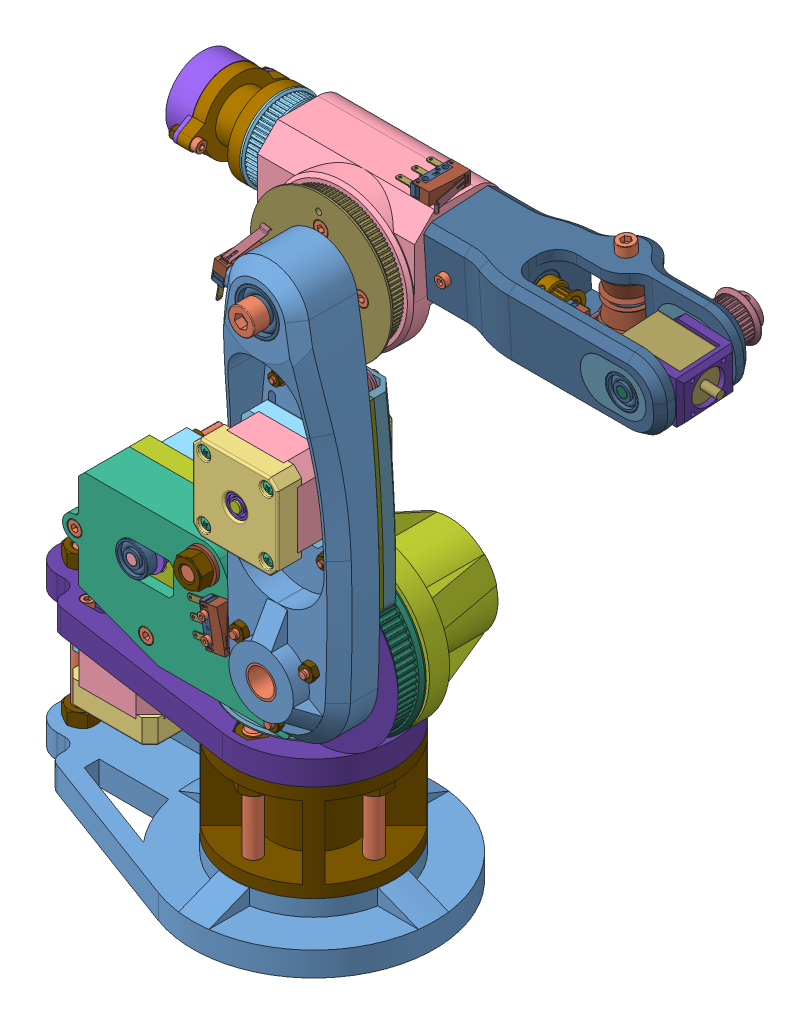
SolidWorks assembly Assem4_v2, configuration Default. Lengths in mm. (continued)
Mates (geometry in assembly coordinates): (continued)
- Coincident177: coincident: plane of Pulley100TBase-2 through (106.8987 -12.6787 52.4417) normal (0 -1 0); plane of thrust ball bearing_68_iso-1 through (106.6815 -12.6787 62.7394) normal (0 1 0)
- Coincident178: coincident: plane of Baseplate-1 through (106.8987 -29.6787 52.4417) normal (0 -1 0); plane of NEMA 17 kiinalaiset-2/Tapa-1 through (25.5987 -29.6787 52.4417) normal (0 1 0)
- Concentric171: concentric: cylinder of Baseplate-1 through (10.0987 -41.6995 36.9417) axis (0 1 0) radius 1.75; cylinder of NEMA 17 kiinalaiset-2/Tapa-1 through (10.0987 -34.1787 36.9417) axis (0 1 0) radius 1.5
- Concentric172: concentric: cylinder of Baseplate-1 through (41.0987 -41.6995 67.9417) axis (0 1 0) radius 1.75; cylinder of NEMA 17 kiinalaiset-2/Tapa-1 through (41.0987 -34.1787 67.9417) axis (0 1 0) radius 1.5
- Concentric173: concentric: cylinder of Baseplate-1 through (10.0987 -41.6995 36.9417) axis (0 1 0) radius 1.75; cylinder of socket head cap screw_iso-60 through (10.0987 12.0713 36.9417) axis (0 1 0) radius 2.75
- Coincident179: coincident: plane of Baseplate-1 through (18.0987 -22.6787 36.9417) normal (0 1 0); plane of socket head cap screw_iso-60 through (12.7426 -22.6787 36.1851) normal (0 -1 0)
- Concentric174: concentric: cylinder of Baseplate-1 through (10.0987 -41.6995 67.9417) axis (0 1 0) radius 1.75; cylinder of socket head cap screw_iso-61 through (10.0987 12.0713 67.9417) axis (0 1 0) radius 2.75
- Coincident180: coincident: plane of Baseplate-1 through (18.0987 -22.6787 67.9417) normal (0 1 0); plane of socket head cap screw_iso-61 through (12.8487 -22.6787 67.9417) normal (0 -1 0)
- Concentric175: concentric: cylinder of Baseplate-1 through (41.0987 -22.6787 36.9417) axis (0 1 0) radius 3; cylinder of socket head cap screw_iso-62 through (41.0987 12.0713 36.9417) axis (0 1 0) radius 2.75
- Coincident181: coincident: plane of Baseplate-1 through (49.0987 -22.6787 36.9417) normal (0 1 0); plane of socket head cap screw_iso-62 through (43.8487 -22.6787 36.9417) normal (0 -1 0)
- Concentric176: concentric: cylinder of Baseplate-1 through (41.0987 -22.6787 67.9417) axis (0 1 0) radius 3; cylinder of socket head cap screw_iso-63 through (41.0987 12.0713 67.9417) axis (0 1 0) radius 2.75
- Coincident182: coincident: plane of Baseplate-1 through (49.0987 -22.6787 67.9417) normal (0 1 0); plane of socket head cap screw_iso-63 through (43.8487 -22.6787 67.9417) normal (0 -1 0)
- Concentric177: concentric: cylinder of NEMA 17 kiinalaiset-2/Eje-1 through (25.5987 -7.6787 52.4417) axis (0 -1 0) radius 2.5; cylinder of GT2_16T_13x14-3 through (25.5987 -20.2487 52.4417) axis (0 1 0) radius 2.5
- Coincident183: coincident: plane of Pulley100TBase-2 through (106.8987 -14.0787 52.4417) normal (0 1 0); plane of GT2_16T_13x14-3 through (25.5987 -14.0787 52.4417) normal (0 1 0)
- Concentric178: concentric: cylinder of Bottom support-1 through (106.8987 -110.9924 22.4417) axis (0 1 0) radius 4; cylinder of socket head cap screw_iso-65 through (106.8987 -129.4287 22.4417) axis (0 -1 0) radius 6.5
- Coincident184: coincident: plane of Bottom support-1 through (106.8987 -89.6787 22.4417) normal (0 -1 0); plane of socket head cap screw_iso-65 through (100.3987 -89.6787 22.4417) normal (0 1 0)
- Concentric179: concentric: cylinder of Bottom support-1 through (76.8987 -89.6787 52.4417) axis (0 -1 0) radius 7.5; cylinder of socket head cap screw_iso-66 through (76.8987 -129.4287 52.4417) axis (0 -1 0) radius 6.5
- Coincident185: coincident: plane of Bottom support-1 through (76.8987 -89.6787 52.4417) normal (0 -1 0); plane of socket head cap screw_iso-66 through (70.3987 -89.6787 52.4417) normal (0 1 0)
- Concentric180: concentric: cylinder of Bottom support-1 through (106.8987 -110.9924 82.4417) axis (0 1 0) radius 4; cylinder of socket head cap screw_iso-67 through (106.8987 -129.4287 82.4417) axis (0 -1 0) radius 6.5
- Coincident186: coincident: plane of Bottom support-1 through (106.8987 -89.6787 82.4417) normal (0 -1 0); plane of socket head cap screw_iso-67 through (100.3987 -89.6787 82.4417) normal (0 1 0)
- Concentric181: concentric: cylinder of Bottom support-1 through (136.8987 -110.9924 52.4417) axis (0 1 0) radius 4; cylinder of socket head cap screw_iso-68 through (136.8987 -129.4287 52.4417) axis (0 -1 0) radius 6.5
- Coincident187: coincident: plane of Bottom support-1 through (136.8987 -89.6787 52.4417) normal (0 -1 0); plane of socket head cap screw_iso-68 through (130.3987 -89.6787 52.4417) normal (0 1 0)
- Concentric182: concentric: cylinder of socket head cap screw_iso-65 through (106.8987 -129.4287 22.4417) axis (0 -1 0) radius 4; cylinder of hex nut style 1 gradeab_iso-26 through (106.8987 -19.4412 22.4417) axis (0 -1 0) radius 4
- Concentric183: concentric: cylinder of socket head cap screw_iso-68 through (136.8987 -129.4287 52.4417) axis (0 -1 0) radius 4; cylinder of hex nut style 1 gradeab_iso-27 through (136.8987 -19.4412 52.4417) axis (0 -1 0) radius 4
- Concentric184: concentric: cylinder of socket head cap screw_iso-67 through (106.8987 -129.4287 82.4417) axis (0 -1 0) radius 4; cylinder of hex nut style 1 gradeab_iso-28 through (106.8987 -19.4412 82.4417) axis (0 -1 0) radius 4
- Concentric185: concentric: cylinder of socket head cap screw_iso-66 through (76.8987 -129.4287 52.4417) axis (0 -1 0) radius 4; cylinder of hex nut style 1 gradeab_iso-29 through (76.8987 -18.4412 52.4417) axis (0 -1 0) radius 4
- Concentric186: concentric: cylinder of Baseplate-1 through (106.8987 -42.9924 82.4417) axis (0 1 0) radius 4; cylinder of hex nut style 1 gradeab_iso-30 through (106.8987 -45.9162 82.4417) axis (0 1 0) radius 4
- Coincident188: coincident: plane of Baseplate-1 through (106.8987 -27.6787 52.4417) normal (0 1 0); plane of hex nut style 1 gradeab_iso-30 through (103.146 -27.6787 75.9417) normal (0 -1 0)
- Concentric187: concentric: cylinder of socket head cap screw_iso-68 through (136.8987 -129.4287 52.4417) axis (0 -1 0) radius 4; cylinder of hex nut style 1 gradeab_iso-31 through (136.8987 -2.6412 52.4417) axis (0 -1 0) radius 4
- Concentric188: concentric: cylinder of Baseplate-1 through (106.8987 -42.9924 22.4417) axis (0 1 0) radius 4; cylinder of hex nut style 1 gradeab_iso-32 through (106.8987 -45.9162 22.4417) axis (0 1 0) radius 4
- Coincident189: coincident: plane of Baseplate-1 through (106.8987 -27.6787 52.4417) normal (0 1 0); plane of hex nut style 1 gradeab_iso-32 through (110.6515 -27.6787 28.9417) normal (0 -1 0)
- Concentric189: concentric: cylinder of socket head cap screw_iso-66 through (76.8987 -129.4287 52.4417) axis (0 -1 0) radius 4; cylinder of hex nut style 1 gradeab_iso-33 through (76.8987 -2.6412 52.4417) axis (0 -1 0) radius 4
- Coincident190: coincident: plane of Bottom Tube-1 through (106.8987 -37.6787 52.4417) normal (0 -1 0); plane of hex nut style 1 gradeab_iso-28 through (106.8987 -37.6787 89.9473) normal (0 1 0)
- Coincident191: coincident: plane of hex nut style 1 gradeab_iso-26 through (106.8987 -37.6787 29.9473) normal (0 1 0); plane of Bottom Tube-1 through (106.8987 -37.6787 52.4417) normal (0 -1 0)
- Coincident192: coincident: plane of Bottom Tube-1 through (106.8987 -37.6787 52.4417) normal (0 -1 0); plane of hex nut style 1 gradeab_iso-27 through (136.8987 -37.6787 59.9473) normal (0 1 0)
- Coincident193: coincident: plane of Baseplate-1 through (143.3987 -27.6787 56.1945) normal (-1 0 0); plane of hex nut style 1 gradeab_iso-31 through (143.3987 -20.8787 56.1945) normal (1 0 0)
- Coincident194: coincident: plane of Baseplate-1 through (106.8987 -27.6787 52.4417) normal (0 1 0); plane of hex nut style 1 gradeab_iso-31 through (136.8987 -27.6787 59.9473) normal (0 -1 0)
- Coincident195: coincident: plane of Baseplate-1 through (114.4043 -27.6787 22.4417) normal (-0.866025 0 0.5); plane of hex nut style 1 gradeab_iso-32 through (114.4043 -27.6787 22.4417) normal (0.866025 0 -0.5)
- Coincident196: coincident: plane of Baseplate-1 through (70.3987 -27.6787 56.1945) normal (0.5 0 -0.866025); plane of hex nut style 1 gradeab_iso-33 through (76.8987 -20.8787 59.9473) normal (-0.5 0 0.866025)
- Coincident197: coincident: plane of Baseplate-1 through (106.8987 -27.6787 52.4417) normal (0 1 0); plane of hex nut style 1 gradeab_iso-33 through (76.8987 -27.6787 59.9473) normal (0 -1 0)
- Coincident198: coincident: plane of Baseplate-1 through (103.146 -27.6787 75.9417) normal (0.866025 0 0.5); plane of hex nut style 1 gradeab_iso-30 through (103.146 -27.6787 75.9417) normal (-0.866025 0 -0.5)
- Concentric190: concentric: cylinder of Nema 14 stepper-1 through (113.8987 155.7922 35.8417) axis (-1 0 0) radius 1.5; cylinder of socket head cap screw_iso-42 through (69.6487 155.7922 35.8417) axis (-1 0 0) radius 1.5
- Concentric191: concentric: cylinder of Bottom support-1 through (-8.1013 -75.7993 52.4417) axis (0 -1 0) radius 4.2; cylinder of hex bolt gradeab_iso-2 through (-8.1013 -98.9787 52.4417) axis (0 -1 0) radius 6.5
- Coincident201: coincident: plane of Bottom support-1 through (106.8987 -93.6787 52.4417) normal (0 -1 0); plane of hex bolt gradeab_iso-2 through (-15.6068 -93.6787 52.4417) normal (0 1 0)
- Coincident202: coincident: plane of Bottom support-1 through (-11.854 -93.6787 45.9417) normal (0 0 1); plane of hex bolt gradeab_iso-2 through (-11.854 -93.6787 45.9417) normal (0 0 -1)
- Concentric192: concentric: cylinder of hex bolt gradeab_iso-2 through (-8.1013 -98.9787 52.4417) axis (0 -1 0) radius 4; cylinder of hex nut style 1 gradeab_iso-35 through (-8.1013 -62.6412 52.4417) axis (0 -1 0) radius 4
- Concentric193: concentric: cylinder of hex bolt gradeab_iso-2 through (-8.1013 -98.9787 52.4417) axis (0 -1 0) radius 4; cylinder of hex nut style 1 gradeab_iso-36 through (-8.1013 -13.4412 52.4417) axis (0 -1 0) radius 4
- Concentric194: concentric: cylinder of hex bolt gradeab_iso-2 through (-8.1013 -98.9787 52.4417) axis (0 -1 0) radius 4; cylinder of hex nut style 1 gradeab_iso-37 through (-8.1013 5.3588 52.4417) axis (0 -1 0) radius 4
- Coincident203: coincident: plane of Bottom support-1 through (106.8987 -87.6787 52.4417) normal (0 1 0); plane of hex nut style 1 gradeab_iso-35 through (-8.1013 -87.6787 59.9473) normal (0 -1 0)
- Coincident204: coincident: plane of Baseplate-1 through (106.8987 -19.6787 52.4417) normal (0 1 0); plane of hex nut style 1 gradeab_iso-37 through (-8.1013 -19.6787 59.9473) normal (0 -1 0)
- Coincident206: coincident: plane of Baseplate-1 through (106.8987 -31.6787 52.4417) normal (0 -1 0); plane of hex nut style 1 gradeab_iso-36 through (-8.1013 -31.6787 59.9473) normal (0 1 0)
- Concentric196: concentric: cylinder of Nema 17 planetary 5 to 1 gearbox-1 through (59.3987 35.6213 65.4417) axis (0 0 -1) radius 3; cylinder of HTD pulley adapter-1 through (59.3987 35.6213 65.4417) axis (0 0 -1) radius 3
- Coincident208: coincident: plane of Nema 17 planetary 5 to 1 gearbox-1 through (59.3987 35.6213 65.4417) normal (0 0 1); plane of HTD pulley adapter-1 through (59.3987 35.6213 65.4417) normal (0 0 -1)
- Concentric200: concentric: cylinder of Nema 17 planetary 5 to 1 gearbox-1 through (59.3987 35.6213 49.4417) axis (0 0 -1) radius 11; cylinder of Motor1 spacer-1 through (59.3987 35.6213 62.4417) axis (0 0 -1) radius 9
- Concentric201: concentric: cylinder of Nema 17 planetary 5 to 1 gearbox-1 through (49.4992 45.5208 42.4417) axis (0 0 1) radius 1.5; cylinder of Motor1 spacer-1 through (49.4992 45.5208 42.7748) axis (0 0 1) radius 1.65
- Coincident214: coincident: plane of Nema 17 planetary 5 to 1 gearbox-1 through (59.3987 35.6213 47.4417) normal (0 0 1); plane of Motor1 spacer-1 through (59.3987 35.6213 47.4417) normal (0 0 -1)
- Concentric202: concentric: cylinder of Motor1 spacer-1 through (49.4992 45.5208 42.7748) axis (0 0 1) radius 1.65; cylinder of socket head cap screw_iso-70 through (49.4992 45.5208 89.1917) axis (0 0 1) radius 2.75
- Coincident215: coincident: plane of Motor1 spacer-1 through (59.3987 35.6213 54.4417) normal (0 0 1); plane of socket head cap screw_iso-70 through (49.4992 48.2708 54.4417) normal (0 0 -1)
- Concentric203: concentric: cylinder of Motor1 spacer-1 through (69.2982 45.5208 42.7748) axis (0 0 1) radius 1.65; cylinder of socket head cap screw_iso-71 through (69.2982 45.5208 89.1917) axis (0 0 1) radius 2.75
- Coincident216: coincident: plane of Motor1 spacer-1 through (59.3987 35.6213 54.4417) normal (0 0 1); plane of socket head cap screw_iso-71 through (69.2982 48.2708 54.4417) normal (0 0 -1)
- Concentric204: concentric: cylinder of Motor1 spacer-1 through (69.2982 25.7218 42.7748) axis (0 0 1) radius 1.65; cylinder of socket head cap screw_iso-72 through (69.2982 25.7218 89.1917) axis (0 0 1) radius 2.75
- Coincident217: coincident: plane of Motor1 spacer-1 through (59.3987 35.6213 54.4417) normal (0 0 1); plane of socket head cap screw_iso-72 through (69.2982 28.4718 54.4417) normal (0 0 -1)
- Concentric205: concentric: cylinder of Motor1 spacer-1 through (49.4992 25.7218 42.7748) axis (0 0 1) radius 1.65; cylinder of socket head cap screw_iso-73 through (49.4992 25.7218 89.1917) axis (0 0 1) radius 2.75
- Coincident218: coincident: plane of Motor1 spacer-1 through (59.3987 35.6213 54.4417) normal (0 0 1); plane of socket head cap screw_iso-73 through (49.4992 28.4718 54.4417) normal (0 0 -1)
- Concentric212: concentric: cylinder of Motor1 spacer-1 through (76.8987 53.1213 62.4417) axis (0 0 -1) radius 2; cylinder of hex nut style 1 gradeab_iso-39 through (76.8987 53.1213 69.2792) axis (0 0 -1) radius 2
- Coincident226: coincident: plane of Motor1 spacer-1 through (59.3987 35.6213 47.4417) normal (0 0 -1); plane of hex nut style 1 gradeab_iso-39 through (78.4468 49.3881 47.4417) normal (0 0 1)
- Concentric213: concentric: cylinder of Motor1 spacer-1 through (41.8987 53.1213 62.4417) axis (0 0 -1) radius 2; cylinder of hex nut style 1 gradeab_iso-40 through (41.8987 53.1213 69.2792) axis (0 0 -1) radius 2
- Coincident227: coincident: plane of Motor1 spacer-1 through (59.3987 35.6213 47.4417) normal (0 0 -1); plane of hex nut style 1 gradeab_iso-40 through (43.4468 49.3881 47.4417) normal (0 0 1)
- Concentric214: concentric: cylinder of Motor1 spacer-1 through (41.8987 18.1213 62.4417) axis (0 0 -1) radius 2; cylinder of hex nut style 1 gradeab_iso-41 through (41.8987 18.1213 69.2792) axis (0 0 -1) radius 2
- Coincident228: coincident: plane of Motor1 spacer-1 through (59.3987 35.6213 47.4417) normal (0 0 -1); plane of hex nut style 1 gradeab_iso-41 through (43.4468 14.3881 47.4417) normal (0 0 1)
- Concentric215: concentric: cylinder of Motor1 spacer-1 through (76.8987 18.1213 62.4417) axis (0 0 -1) radius 2; cylinder of hex nut style 1 gradeab_iso-42 through (76.8987 18.1213 69.2792) axis (0 0 -1) radius 2
- Coincident229: coincident: plane of Motor1 spacer-1 through (59.3987 35.6213 47.4417) normal (0 0 -1); plane of hex nut style 1 gradeab_iso-42 through (78.4468 14.3881 47.4417) normal (0 0 1)
- Concentric216: concentric: cylinder of socket head cap screw_iso-54 through (30.3987 34.1213 126.3917) axis (0 0 1) radius 2; cylinder of Basewall cover v2-1 through (30.3987 34.1213 66.7849) axis (0 0 1) radius 2
- Concentric217: concentric: cylinder of socket head cap screw_iso-50 through (65.8987 5.6213 126.3917) axis (0 0 1) radius 2; cylinder of Basewall cover v2-1 through (65.8987 5.6213 94.6417) axis (0 0 -1) radius 2.1
- Coincident231: coincident: plane of socket head cap screw_iso-54 through (29.6963 37.5501 90.6417) normal (0 0 -1); plane of Basewall cover v2-1 through (30.3987 34.1213 90.6417) normal (0 0 1)
- Coincident232: coincident: plane of socket head cap screw_iso-50 through (67.7589 8.5861 90.6417) normal (0 0 -1); plane of Basewall cover v2-1 through (65.8987 5.6213 90.6417) normal (0 0 1)
- Concentric220: concentric: cylinder of socket head cap screw_iso-23 through (94.3987 50.6213 22.6917) axis (0 0 -1) radius 4; cylinder of plain washer normal grade a_iso-20 through (94.3987 50.6213 129.5667) axis (0 0 1) radius 4.2
- Coincident233: coincident: plane of plain washer normal grade a_iso-20 through (90.8481 52.8648 94.6417) normal (0 0 -1); plane of Basewall cover v2-1 through (133.7832 -1.1274 94.6417) normal (0 0 1)
- Concentric221: concentric: cylinder of socket head cap screw_iso-36 through (101.319 35.6213 134.5917) axis (0 0 1) radius 1; cylinder of Basewall cover v2-1 through (101.319 35.6213 86.8133) axis (0 0 1) radius 1
- Concentric222: concentric: cylinder of socket head cap screw_iso-37 through (103.0555 25.7732 134.5917) axis (0 0 1) radius 1; cylinder of Basewall cover v2-1 through (103.0555 25.7732 86.8133) axis (0 0 1) radius 1
- Coincident234: coincident: plane of ? through (103.04 32.6599 94.6417) normal (0 0 -1); plane of Basewall cover v2-1 through (133.7832 -1.1274 94.6417) normal (0 0 1)
- Concentric223: concentric: cylinder of 90mm aluputki-1 through (144.3987 35.6213 116.0417) axis (0 0 -1) radius 7.5; cylinder of BaseWall_2_v2-1 through (144.3987 35.6213 72.4417) axis (0 0 -1) radius 10
- Concentric224: concentric: cylinder of Pulley100TBase-2 through (106.8987 -14.0787 52.4417) axis (0 1 0) radius 7.5; cylinder of BaseWall_2_v2-1 through (106.8987 40.6213 52.4417) axis (0 -1 0) radius 7.65
- Coincident235: coincident: plane of angular contact ball bearing_68_iso-5 through (152.6194 47.2916 63.4417) normal (0 0 -1); plane of BaseWall_2_v2-1 through (144.3987 35.6213 63.4417) normal (0 0 1)
- Coincident236: coincident: plane of angular contact ball bearing_68_iso-6 through (145.4625 51.2852 31.4417) normal (0 0 1); plane of BaseWall_2_v2-1 through (144.3987 35.6213 31.4417) normal (0 0 -1)
- Coincident237: coincident: plane of Bottom spacer-1 through (106.8987 -4.3787 52.4417) normal (0 1 0); plane of BaseWall_2_v2-1 through (144.3987 -4.3787 72.4417) normal (0 -1 0)
- Concentric225: concentric: cylinder of socket head cap screw_iso-58 through (131.8987 -47.4287 52.4417) axis (0 -1 0) radius 2; cylinder of BaseWall_2_v2-1 through (131.8987 5.6213 52.4417) axis (0 -1 0) radius 2
- Coincident238: coincident: plane of Basewall cover v2-1 through (94.3987 50.6213 72.4417) normal (0 0 -1); plane of BaseWall_2_v2-1 through (144.3987 35.6213 72.4417) normal (0 0 1)
- Coincident239: coincident: plane of Basewall cover v2-1 through (32.3987 60.6213 89.6417) normal (-1 0 0); plane of BaseWall_2_v2-1 through (32.3987 60.6213 72.4417) normal (-1 0 0)
- Concentric226: concentric: cylinder of socket head cap screw_iso-23 through (94.3987 50.6213 22.6917) axis (0 0 -1) radius 4; cylinder of BaseWall_2_v2-1 through (94.3987 50.6213 72.4417) axis (0 0 -1) radius 4.1
- Coincident240: coincident: plane of socket head cap screw_iso-23 through (94.477 57.1208 62.4417) normal (0 0 1); plane of BaseWall_2_v2-1 through (144.3987 35.6213 62.4417) normal (0 0 -1)
- Concentric227: concentric: cylinder of socket head cap screw_iso-23 through (94.3987 50.6213 22.6917) axis (0 0 -1) radius 4; cylinder of plain washer normal grade a_iso-17 through (94.3987 50.6213 107.3667) axis (0 0 1) radius 4.2
- Coincident241: coincident: plane of plain washer normal grade a_iso-17 through (94.3987 54.8213 72.4417) normal (0 0 -1); plane of BaseWall_2_v2-1 through (144.3987 35.6213 72.4417) normal (0 0 1)
- Coincident242: coincident: plane of hex nut style 1 gradeab_iso-22 through (33.8987 36.142 67.4417) normal (0 0 1); plane of BaseWall_2_v2-1 through (144.3987 35.6213 67.4417) normal (0 0 -1)
- Coincident243: coincident: plane of Basewall cover v2-1 through (32.3987 60.6213 89.6417) normal (0 1 0); plane of BaseWall_2_v2-1 through (84.3987 60.6213 72.4417) normal (0 1 0); plane of hex nut style 1 gradeab_iso-22; plane of BaseWall_2_v2-1
- Parallel6: parallel: plane of hex nut style 1 gradeab_iso-22 through (33.8987 36.142 64.2417) normal (0.5 0.866025 0); plane of BaseWall_2_v2-1 through (30.3987 38.2782 67.4417) normal (-0.5 -0.866025 0)
- Coincident245: coincident: plane of Motor1 spacer-1 through (59.3987 35.6213 62.4417) normal (0 0 1); plane of BaseWall_2_v2-1 through (144.3987 35.6213 62.4417) normal (0 0 -1)
- Concentric228: concentric: cylinder of Motor1 spacer-1 through (41.8987 53.1213 62.4417) axis (0 0 -1) radius 2; cylinder of socket head cap screw_iso-75 through (41.8987 53.1213 104.1917) axis (0 0 1) radius 2
- Coincident246: coincident: plane of socket head cap screw_iso-75 through (41.8987 56.6213 68.4417) normal (0 0 -1); plane of BaseWall_2_v2-1 through (49.8987 53.1213 68.4417) normal (0 0 1)
- Concentric229: concentric: cylinder of socket head cap screw_iso-75 through (41.8987 53.1213 104.1917) axis (0 0 1) radius 3.5; cylinder of BaseWall_2_v2-1 through (41.8987 53.1213 68.4417) axis (0 0 1) radius 3.7
- Concentric230: concentric: cylinder of Motor1 spacer-1 through (76.8987 53.1213 62.4417) axis (0 0 -1) radius 2; cylinder of socket head cap screw_iso-76 through (76.8987 53.1213 104.1917) axis (0 0 1) radius 2
- Coincident247: coincident: plane of socket head cap screw_iso-76 through (76.8987 56.6213 68.4417) normal (0 0 -1); plane of BaseWall_2_v2-1 through (84.8987 53.1213 68.4417) normal (0 0 1)
- Concentric231: concentric: cylinder of Motor1 spacer-1 through (41.8987 18.1213 62.4417) axis (0 0 -1) radius 2; cylinder of socket head cap screw_iso-77 through (41.8987 18.1213 104.1917) axis (0 0 1) radius 2
- Coincident248: coincident: plane of socket head cap screw_iso-77 through (41.8987 21.6213 68.4417) normal (0 0 -1); plane of BaseWall_2_v2-1 through (41.8987 18.1213 68.4417) normal (0 0 1)
- Concentric232: concentric: cylinder of socket head cap screw_iso-77 through (41.8987 18.1213 104.1917) axis (0 0 1) radius 3.5; cylinder of BaseWall_2_v2-1 through (41.8987 18.1213 68.4417) axis (0 0 1) radius 3.7
- Concentric233: concentric: cylinder of Motor1 spacer-1 through (76.8987 18.1213 62.4417) axis (0 0 -1) radius 2; cylinder of socket head cap screw_iso-78 through (76.8987 18.1213 104.1917) axis (0 0 1) radius 2
- Coincident249: coincident: plane of socket head cap screw_iso-78 through (76.8987 21.6213 68.4417) normal (0 0 -1); plane of BaseWall_2_v2-1 through (84.8987 18.1213 68.4417) normal (0 0 1)
- Coincident250: coincident: plane of hex nut style 1 gradeab_iso-21 through (69.3494 3.5175 62.4417) normal (0 0 1); plane of BaseWall_2_v2-1 through (144.3987 35.6213 62.4417) normal (0 0 -1)
- Concentric237: concentric: cylinder of hex nut style 1 gradeab_iso-23 through (106.8987 49.4213 52.4417) axis (0 -1 0) radius 3.4; cylinder of BaseWall_2_v2-1 through (106.8987 40.6213 52.4417) axis (0 -1 0) radius 7.65; plane of hex nut style 1 gradeab_iso-23; plane of BaseWall_2_v2-1; plane of hex nut style 1 gradeab_iso-23; plane of BaseWall_2_v2-1
- Distance3: distance = 2 mm: plane of hex nut style 1 gradeab_iso-23 through (110.6515 42.6213 58.9417) normal (0 -1 0); plane of BaseWall_2_v2-1 through (106.8987 40.6213 52.4417) normal (0 1 0)
- Parallel7: parallel: plane of hex nut style 1 gradeab_iso-23 through (110.6515 49.4213 58.9417) normal (0 0 1); plane of BaseWall_2_v2-1 through (144.3987 35.6213 62.4417) normal (0 0 -1)
- Concentric238: concentric: cylinder of HTD pulley adapter-1 through (59.3987 35.6213 76.4417) axis (0 0 -1) radius 3; cylinder of 3M HTD 16T 6mm Bore-1 through (59.3987 35.6213 76.2417) axis (0 0 -1) radius 3
- Coincident253: coincident: plane of HTD3M 80T-1 through (144.3987 35.6213 76.2417) normal (0 0 1); plane of 3M HTD 16T 6mm Bore-1 through (59.3987 35.6213 76.2417) normal (0 0 1)
- Concentric240: concentric: cylinder of HTD pulley adapter-1 through (59.3987 35.6213 95.4417) axis (0 0 -1) radius 2.5; cylinder of angular contact ball bearing_68_iso-11 through (59.3987 35.6213 113.5792) axis (0 0 -1) radius 2.5
- Coincident254: coincident: plane of HTD pulley adapter-1 through (59.3987 35.6213 90.4417) normal (0 0 1); plane of angular contact ball bearing_68_iso-11 through (56.6269 35.2251 90.4417) normal (0 0 -1)
- Concentric241: concentric: cylinder of 100mm aluputki-1 through (211.1987 210.6213 52.4417) axis (-1 0 0) radius 6.5; cylinder of 6mm akseli-1 through (241.6987 210.6213 52.4417) axis (-1 0 0) radius 2.5
- Coincident260: coincident: plane of Nema 14 Round stepper-2 through (71.6987 210.6213 52.4417) normal (1 0 0); plane of 6mm akseli-1 through (71.6987 210.6213 52.4417) normal (-1 0 0)
- Concentric252: concentric: cylinder of Pulley100TBase-2 through (106.8987 -12.6787 52.4417) axis (0 -1 0) radius 17.5; cylinder of thrust ball bearing_68_iso-1 through (106.8987 17.2463 52.4417) axis (0 -1 0) radius 17.5
- Concentric253: concentric: cylinder of thrust ball bearing_68_iso-1 through (106.8987 -52.6037 52.4417) axis (0 1 0) radius 17.5; cylinder of Baseplate-1 through (106.8987 -22.6787 52.4417) axis (0 1 0) radius 17.65; plane of Arm2Mountv2-1; plane of ?
- Distance14: distance = 2 mm: plane of Arm2Mountv2-1 through (179.3987 195.6213 66.8417) normal (1 0 0); plane of ? through (177.3987 230.6213 51.0917) normal (1 0 0)
- Coincident301: coincident: plane of Arm2Mountv2-1 through (109.3987 230.6213 66.8417) normal (0 1 0); plane of ? through (170.9793 230.6213 56.7514) normal (0 -1 0)
- Concentric262: concentric: cylinder of 100mm aluputki-1 through (211.1987 210.6213 52.4417) axis (-1 0 0) radius 7.5; cylinder of Rotation arm V3-1 through (216.3987 210.6213 52.4417) axis (-1 0 0) radius 7.7
- Coincident306: coincident: plane of angular contact ball bearing_68_iso-3 through (179.3987 212.2986 60.0592) normal (1 0 0); plane of Rotation arm V3-1 through (179.3987 210.6213 52.4417) normal (-1 0 0)
- Concentric263: concentric: cylinder of socket head cap screw_iso-86 through (183.3987 167.075 10.8093) axis (0 -0.758027 -0.652223) radius 1.5; cylinder of Rotation arm V3-1 through (183.3987 203.2709 41.9529) axis (0 -0.758027 -0.652223) radius 1.5
- Distance15: distance = 3 mm: plane of Rotation arm V3-1 through (180.3987 197.3162 33.5413) normal (0 -0.758027 -0.652223); plane of socket head cap screw_iso-86 through (182.6991 191.6819 35.49) normal (0 0.758027 0.652223)
- Concentric264: concentric: cylinder of socket head cap screw_iso-84 through (190.3987 207.2086 105.0812) axis (0 -0.064696 0.997905) radius 1.5; cylinder of Rotation arm V3-1 through (190.3987 212.7563 19.5098) axis (0 -0.064696 0.997905) radius 1.5
- Coincident308: coincident: plane of socket head cap screw_iso-84 through (193.1125 209.0127 70.3752) normal (0 0.064696 -0.997905); plane of Rotation arm V3-1 through (200.3987 262.2014 73.8235) normal (0 -0.064696 0.997905)
- Coincident309: coincident: plane of Motor 5 adapter-1 through (90.1987 210.6213 52.4417) normal (0 0.997905 0.064696); plane of Rotation arm V3-1 through (180.3987 210.6213 52.4417) normal (0 -0.997905 -0.064696)
- Coincident310: coincident: plane of angular contact ball bearing_68_iso-12 through (216.3987 213.4046 46.1553) normal (-1 0 0); plane of Rotation arm V3-1 through (216.3987 210.6213 52.4417) normal (1 0 0)
- Coincident311: coincident: plane of angular contact ball bearing_68_iso-12 through (221.3987 211.7549 49.8814) normal (1 0 0); plane of GT2_16T_13x14-4 through (221.3987 210.6213 52.4417) normal (-1 0 0)
- Concentric269: concentric: cylinder of 6mm akseli-1 through (241.6987 210.6213 52.4417) axis (-1 0 0) radius 2.5; cylinder of angular contact ball bearing_68_iso-12 through (198.2612 210.6213 52.4417) axis (1 0 0) radius 2.5
- Concentric270: concentric: cylinder of 6mm akseli-1 through (241.6987 210.6213 52.4417) axis (-1 0 0) radius 2.5; cylinder of GT2_16T_13x14-4 through (221.3987 210.6213 52.4417) axis (1 0 0) radius 2.5
- Coincident316: coincident: plane of Rotation arm V3-1 through (216.3987 226.5966 76.5257) normal (0 0.997905 0.064696); plane of socket head cap screw_iso-88 through (243.4859 229.6535 29.3756) normal (0 -0.997905 -0.064696)
- Concentric271: concentric: cylinder of Rotation arm V3-1 through (243.3987 229.3786 33.6158) axis (0 -0.997905 -0.064696) radius 2.6; cylinder of socket head cap screw_iso-88 through (243.3987 266.0516 35.9934) axis (0 0.997905 0.064696) radius 2.5
- Concentric272: concentric: cylinder of socket head cap screw_iso-88 through (243.3987 266.0516 35.9934) axis (0 0.997905 0.064696) radius 2.5; cylinder of angular contact ball bearing_68_iso-18 through (243.3987 200.3021 31.7307) axis (0 0.997905 0.064696) radius 2.5
- Concentric273: concentric: cylinder of socket head cap screw_iso-88 through (243.3987 266.0516 35.9934) axis (0 0.997905 0.064696) radius 2.5; cylinder of angular contact ball bearing_68_iso-19 through (243.3987 195.3126 31.4072) axis (0 0.997905 0.064696) radius 2.5
- Concentric274: concentric: cylinder of socket head cap screw_iso-88 through (243.3987 266.0516 35.9934) axis (0 0.997905 0.064696) radius 2.5; cylinder of angular contact ball bearing_68_iso-20 through (243.3987 187.3294 30.8897) axis (0 0.997905 0.064696) radius 2.5
- Concentric275: concentric: cylinder of socket head cap screw_iso-88 through (243.3987 266.0516 35.9934) axis (0 0.997905 0.064696) radius 2.5; cylinder of angular contact ball bearing_68_iso-21 through (243.3987 182.3398 30.5662) axis (0 0.997905 0.064696) radius 2.5
- Coincident317: coincident: plane of angular contact ball bearing_68_iso-18 through (236.7265 218.2944 34.5581) normal (0 -0.997905 -0.064696); plane of angular contact ball bearing_68_iso-19 through (235.9469 218.2762 34.839) normal (0 0.997905 0.064696)
- Coincident318: coincident: plane of angular contact ball bearing_68_iso-20 through (236.7753 205.3096 33.9021) normal (0 -0.997905 -0.064696); plane of angular contact ball bearing_68_iso-21 through (235.931 205.3074 33.9362) normal (0 0.997905 0.064696)
- Concentric276: concentric: cylinder of socket head cap screw_iso-88 through (243.3987 266.0516 35.9934) axis (0 0.997905 0.064696) radius 2.5; cylinder of plain washer normal grade a_iso-24 through (243.3987 234.2933 33.9344) axis (0 0.997905 0.064696) radius 2.65
- Concentric277: concentric: cylinder of socket head cap screw_iso-88 through (243.3987 266.0516 35.9934) axis (0 0.997905 0.064696) radius 2.5; cylinder of plain washer normal grade a_iso-25 through (243.3987 258.243 35.4871) axis (0 0.997905 0.064696) radius 2.65
- Coincident319: coincident: plane of Rotation arm V3-1 through (180.3987 198.1475 51.633) normal (0 0.997905 0.064696); plane of plain washer normal grade a_iso-24 through (246.0486 199.4431 31.6492) normal (0 -0.997905 -0.064696)
- Coincident320: coincident: plane of Rotation arm V3-1 through (180.3987 223.0951 53.2504) normal (0 -0.997905 -0.064696); plane of plain washer normal grade a_iso-25 through (248.3985 224.3922 33.2438) normal (0 0.997905 0.064696)
- Coincident321: coincident: plane of angular contact ball bearing_68_iso-18 through (240.6813 223.3475 33.9012) normal (0 0.997905 0.064696); plane of plain washer normal grade a_iso-25 through (246.0486 223.3928 33.2019) normal (0 -0.997905 -0.064696)
- Coincident322: coincident: plane of angular contact ball bearing_68_iso-21 through (239.3739 200.3739 32.7491) normal (0 -0.997905 -0.064696); plane of plain washer normal grade a_iso-24 through (248.3985 200.4425 31.6911) normal (0 0.997905 0.064696)
- Concentric278: concentric: cylinder of angular contact ball bearing_68_iso-18 through (243.3987 200.3021 31.7307) axis (0 0.997905 0.064696) radius 8; cylinder of GT2 hihna chamfer rulla-1 through (243.3987 221.8943 33.1306) axis (0 -0.997905 -0.064696) radius 8.25
- Coincident323: coincident: plane of angular contact ball bearing_68_iso-18 through (235.9259 223.271 35.0801) normal (0 0.997905 0.064696); plane of GT2 hihna chamfer rulla-1 through (243.3987 223.3911 33.2276) normal (0 0.997905 0.064696)
- Concentric279: concentric: cylinder of angular contact ball bearing_68_iso-20 through (243.3987 187.3294 30.8897) axis (0 0.997905 0.064696) radius 8; cylinder of GT2 hihna chamfer rulla-2 through (243.3987 201.9362 31.8366) axis (0 0.997905 0.064696) radius 8.25
- Coincident324: coincident: plane of angular contact ball bearing_68_iso-20 through (235.9805 210.2848 34.4462) normal (0 0.997905 0.064696); plane of GT2 hihna chamfer rulla-2 through (243.3987 210.4184 32.3866) normal (0 0.997905 0.064696)
- Coincident328: coincident: plane of Rotation arm V3-1 through (301.3987 192.1875 66.2781) normal (0 0.064696 -0.997905); plane of ? through (247.9793 215.0492 67.7603) normal (0 -0.064696 0.997905)
- Distance16: distance = 4 mm: plane of ? through (253.5487 223.1226 68.2837) normal (0 0.997905 0.064696); plane of Rotation arm V3-1 through (216.3987 226.5966 76.5257) normal (0 0.997905 0.064696)
- Distance17: distance = 15 mm: plane of ? through (244.3987 198.3189 60.8634) normal (-1 0 0); line of Rotation arm V3-1 through (229.3987 213.9128 67.6866) axis (0 0.997905 0.064696)
- Coincident332: coincident: line of Arm2Mountv2-1 through (144.3987 230.6213 64.8417) axis (1 0 0); plane of ? through (176.5487 230.6213 64.8417) normal (0 0 1)
- Concentric284: concentric: cylinder of Pulley100TBase-2 through (106.8987 -14.0787 52.4417) axis (0 1 0) radius 7.5; cylinder of Bottom spacer-1 through (106.8987 -6.3787 52.4417) axis (0 1 0) radius 7.5
- Concentric285: concentric: cylinder of bearing adapter J6 housing-1 through (282.7987 209.6509 67.4103) axis (0 -0.064696 0.997905) radius 8.2; cylinder of angular contact ball bearing_68_iso-23 through (282.7987 207.9599 93.493) axis (0 0.064696 -0.997905) radius 8
- Coincident333: coincident: plane of bearing adapter J6 housing-1 through (282.7987 209.4568 70.404) normal (0 -0.064696 0.997905); plane of angular contact ball bearing_68_iso-23 through (279.9117 202.3335 69.9422) normal (0 0.064696 -0.997905)
- Concentric286: concentric: cylinder of angular contact ball bearing_68_iso-22 through (282.7987 213.2827 11.3904) axis (0 -0.064696 0.997905) radius 8; cylinder of bearing adapter J6 housing-2 through (282.7987 211.5918 37.4731) axis (0 0.064696 -0.997905) radius 8.2
- Coincident334: coincident: plane of angular contact ball bearing_68_iso-22 through (278.5959 205.3475 34.062) normal (0 -0.064696 0.997905); plane of bearing adapter J6 housing-2 through (282.7987 211.7858 34.4794) normal (0 0.064696 -0.997905)
- Concentric287: concentric: cylinder of Rotation arm V3-1 through (273.3987 206.585 114.7003) axis (0 0.064696 -0.997905) radius 11.2; cylinder of bearing adapter J6 housing-1 through (273.3987 209.6509 67.4103) axis (0 -0.064696 0.997905) radius 11.1
- Coincident335: coincident: plane of Rotation arm V3-1 through (216.3987 191.67 74.2613) normal (0 -0.064696 0.997905); plane of bearing adapter J6 housing-1 through (283.6987 209.1333 75.3935) normal (0 -0.064696 0.997905)
- Concentric288: concentric: cylinder of Rotation arm V3-1 through (273.3987 206.585 114.7003) axis (0 0.064696 -0.997905) radius 11.2; cylinder of bearing adapter J6 housing-2 through (273.3987 211.5918 37.4731) axis (0 0.064696 -0.997905) radius 11.1
- Parallel8: parallel: plane of Rotation arm V3-1 through (273.3987 195.4084 113.9757) normal (0 0.997905 0.064696); plane of bearing adapter J6 housing-1 through (283.6987 198.5741 66.6922) normal (0 -0.997905 -0.064696)
- Parallel9: parallel: plane of Rotation arm V3-1 through (273.3987 195.4084 113.9757) normal (0 0.997905 0.064696); plane of bearing adapter J6 housing-2 through (283.6987 200.515 36.755) normal (0 -0.997905 -0.064696)
- Coincident338: coincident: plane of Rotation arm V3-1 through (216.3987 194.646 28.3577) normal (0 0.064696 -0.997905); plane of bearing adapter J6 housing-2 through (283.6987 212.1093 29.4899) normal (0 0.064696 -0.997905)
- Concentric291: concentric: cylinder of angular contact ball bearing_68_iso-22 through (282.7987 213.2827 11.3904) axis (0 -0.064696 0.997905) radius 2.5; cylinder of 5mm akseli 1-1 through (282.7987 211.2683 42.4627) axis (0 0.064696 -0.997905) radius 2.5
- Concentric293: concentric: cylinder of Pulley32TGT2-1 through (282.7987 212.2387 27.4941) axis (0 -0.064696 0.997905) radius 2.55; cylinder of 5mm akseli 1-1 through (282.7987 211.2683 42.4627) axis (0 0.064696 -0.997905) radius 2.5
- Concentric294: concentric: cylinder of Pulley32TGT2-1 through (280.3133 201.8427 14.2938) axis (0.216125 0.97432 0.063167) radius 1.5; cylinder of 5mm akseli 1-1 through (283.339 215.4832 15.1782) axis (-0.216125 -0.97432 -0.063167) radius 1.5
- Width2: width: plane of J6 kotelo-2 through (272.2958 199.2168 65.7317) normal (0 -0.064696 0.997905); plane of J6 kotelo-2 through (272.2958 201.0283 37.7904) normal (0 0.064696 -0.997905); plane of bearing adapter J6 housing-1 through (283.6987 209.6509 67.4103) normal (0 0.064696 -0.997905); plane of bearing adapter J6 housing-2 through (283.6987 211.5918 37.4731) normal (0 -0.064696 0.997905)
- Coincident342: coincident: plane of 5mm akseli 1-1 through (282.7987 211.2683 42.4627) normal (0 -0.064696 0.997905); plane of J6 kotelo-2 through (272.2958 200.7695 41.782) normal (0 -0.064696 0.997905)
- Concentric297: concentric: cylinder of 5mm akseli 2-1 through (282.7987 209.9744 62.4208) axis (0 -0.064696 0.997905) radius 2.5; cylinder of J6 kotelo-2 through (282.7987 211.9845 31.4148) axis (0 -0.064696 0.997905) radius 2.5
- Coincident343: coincident: plane of 5mm akseli 2-1 through (282.7987 209.9744 62.4208) normal (0 0.064696 -0.997905); plane of J6 kotelo-2 through (272.2958 199.4756 61.7401) normal (0 0.064696 -0.997905)
- Concentric298: concentric: cylinder of Nema8 Stepperi (banggood.com)-1 through (296.1443 217.1926 60.5839) axis (0.998908 -0.046619 -0.003022) radius 1; cylinder of J6 kotelo-2 through (296.3156 217.1846 60.5834) axis (0.998908 -0.046619 -0.003022) radius 1
- Concentric299: concentric: cylinder of Nema8 Stepperi (banggood.com)-1 through (295.4248 202.838 44.2209) axis (0.998908 -0.046619 -0.003022) radius 1; cylinder of J6 kotelo-2 through (295.5962 202.83 44.2204) axis (0.998908 -0.046619 -0.003022) radius 1
- Coincident344: coincident: plane of Nema8 Stepperi (banggood.com)-1 through (298.7813 209.8754 52.3933) normal (0.998908 -0.046619 -0.003022); plane of J6 kotelo-2 through (299.2951 221.4873 43.1252) normal (-0.998908 0.046619 0.003022)
- Concentric300: concentric: cylinder of 5mm akseli 1-1 through (282.7987 211.2683 42.4627) axis (0 0.064696 -0.997905) radius 2.5; cylinder of J6 kotelo-2 through (282.7987 211.9845 31.4148) axis (0 -0.064696 0.997905) radius 2.5
- Concentric301: concentric: cylinder of Pulley60Tv2-1 through (105.1485 221.8919 42.5435) axis (-1 0 0) radius 1.75; cylinder of Motor 5 adapter-1 through (79.249 221.8919 42.5435) axis (1 0 0) radius 1.75
